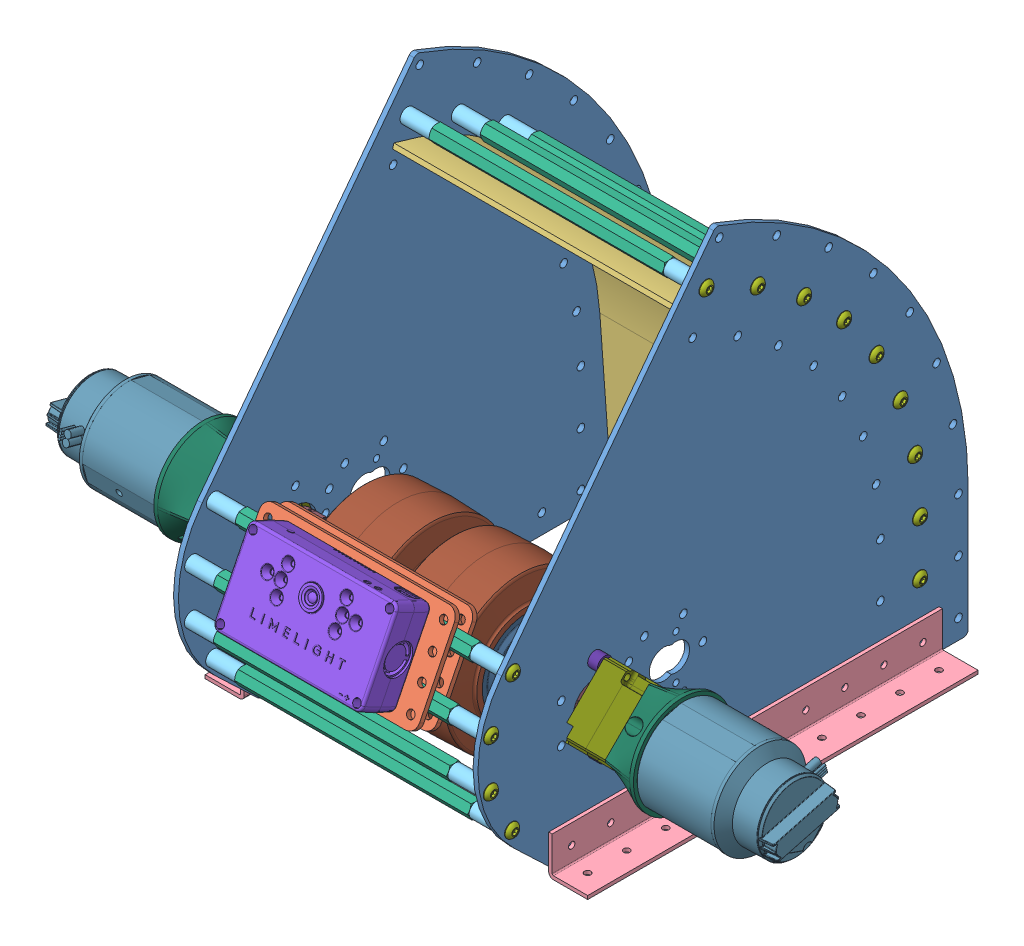
SolidWorks assembly Shooter, configuration Default. Lengths in mm.
Overall size (762 1050.2 1114.79).
114 component instances, 18 part files, 6 mates.
Components (placement in the parent):
- Skeleton-1: Skeleton [Default] at origin
- WCP-0281 Rev1 - GreyT Shooter (Falcon VP Direct)-1: WCP-0281 Rev1 - GreyT Shooter (Falcon VP Direct) [Default] at (-0.625 553.3138 -30.7114) size (474.18 324.22 346.91)
  - frame-GreyT Shooter (Falcon VP Direct)-1: frame-GreyT Shooter (Falcon VP Direct) [Default] at (99.05 0 0) size (248.9 311.77 324.97)
    - WCP-0281-001 Rev1-1: WCP-0281-001 Rev1 [Default] at (-1.5875 82.55 -30.1625) size (3.17 311.77 319.09)
    - WCP-0281-001 Rev1-2: WCP-0281-001 Rev1 [Default] at (-196.5125 82.55 -30.1625) size (3.17 311.77 319.09)
    - WCP-0281-005 Rev1-1: WCP-0281-005 Rev1 [Default] at (-98.4446 110.2154 24.9678) x (1 0 0) z (0 0.446198 0.894934) size (127 63.5 3.17)
    - WCP-0281-005 Rev1-2: WCP-0281-005 Rev1 [Default] at (-98.4446 115.8821 36.3334) x (1 0 0) z (0 0.446198 0.894934) size (127 63.5 3.17)
    - polycarb_flex_panel (WCP-0281-006) Rev1-1: polycarb_flex_panel (WCP-0281-006) Rev1 [Default] at (-97.1926 99.11 -45.232) x (1 0 0) z (0 -0.072501 0.997368) size (184.15 254.67 126.03)
    - WCP-0281-004 Rev1-1: WCP-0281-004 Rev1 [Default] at (0 0 -114.3) size (25.4 25.4 254)
    - WCP-0281-004 Rev1-2: WCP-0281-004 Rev1 [Default] at (-198.1 0 -139.7) x (-1 0 0) z (0 0 -1) size (25.4 25.4 254)
    - spacer_assembly^frame-GreyT Shooter (Falcon VP Direct)-1: spacer_assembly^frame-GreyT Shooter (Falcon VP Direct) [Default] at (-3.8 277.1819 -108.5961) x (1 0 0) z (0 0.167761 -0.985828) size (204.43 13.43 13.43)
      - WCP-0217 Rev1-1: WCP-0217 Rev1 [Default] at (-180.975 -4.7625 -5.4993) x (1 0 0) z (0 -0.707903 0.70631) size (19.05 9.5 9.5)
      - 91780A094_ALUM FEM THRDED HEX STANDOFF (1)_91780A094-1: 91780A094_ALUM FEM THRDED HEX STANDOFF (1)_91780A094 [Default] at (-95.25 -4.7625 -5.4993) x (0 -1 0) z (-1 0 0) size (9.53 11 152.4)
      - WCP-0217 Rev1-2: WCP-0217 Rev1 [Default] at (-9.525 -4.7625 -5.4993) x (1 0 0) z (0 -0.707903 0.70631) size (19.05 9.5 9.5)
      - WCP-0256 Rev1-1: WCP-0256 Rev1 [Default] at (-196.8654 -4.7625 -5.4993) x (0 -0.959732 -0.280918) z (-1 0 0) size (9.24 9.28 34.97)
      - WCP-0256 Rev1-2: WCP-0256 Rev1 [Default] at (6.3654 -4.7625 -5.4993) x (0 0.566489 -0.82407) z (1 0 0) size (9.24 9.28 34.97)
    - spacer_assembly^frame-GreyT Shooter (Falcon VP Direct)-2: spacer_assembly^frame-GreyT Shooter (Falcon VP Direct) [Default] at (-3.8 258.4844 -133.4749) x (1 0 0) z (0 -0.921698 -0.387907) size (204.43 13.43 13.43)
      - WCP-0217 Rev1-1: WCP-0217 Rev1 [Default] at (-180.975 -4.7625 -5.4993) x (1 0 0) z (0 -0.707903 0.70631) size (19.05 9.5 9.5)
      - 91780A094_ALUM FEM THRDED HEX STANDOFF (1)_91780A094-1: 91780A094_ALUM FEM THRDED HEX STANDOFF (1)_91780A094 [Default] at (-95.25 -4.7625 -5.4993) x (0 -1 0) z (-1 0 0) size (9.53 11 152.4)
      - WCP-0217 Rev1-2: WCP-0217 Rev1 [Default] at (-9.525 -4.7625 -5.4993) x (1 0 0) z (0 -0.707903 0.70631) size (19.05 9.5 9.5)
      - WCP-0256 Rev1-1: WCP-0256 Rev1 [Default] at (-196.8654 -4.7625 -5.4993) x (0 -0.959732 -0.280918) z (-1 0 0) size (9.24 9.28 34.97)
      - WCP-0256 Rev1-2: WCP-0256 Rev1 [Default] at (6.3654 -4.7625 -5.4993) x (0 0.566489 -0.82407) z (1 0 0) size (9.24 9.28 34.97)
    - spacer_assembly^frame-GreyT Shooter (Falcon VP Direct)-3: spacer_assembly^frame-GreyT Shooter (Falcon VP Direct) [Default] at (-3.8 237.3746 -163.6227) x (1 0 0) z (0 -0.921698 -0.387907) size (204.43 13.43 13.43)
      - WCP-0217 Rev1-1: WCP-0217 Rev1 [Default] at (-180.975 -4.7625 -5.4993) x (1 0 0) z (0 -0.707903 0.70631) size (19.05 9.5 9.5)
      - 91780A094_ALUM FEM THRDED HEX STANDOFF (1)_91780A094-1: 91780A094_ALUM FEM THRDED HEX STANDOFF (1)_91780A094 [Default] at (-95.25 -4.7625 -5.4993) x (0 -1 0) z (-1 0 0) size (9.53 11 152.4)
      - WCP-0217 Rev1-2: WCP-0217 Rev1 [Default] at (-9.525 -4.7625 -5.4993) x (1 0 0) z (0 -0.707903 0.70631) size (19.05 9.5 9.5)
      - WCP-0256 Rev1-1: WCP-0256 Rev1 [Default] at (-196.8654 -4.7625 -5.4993) x (0 -0.959732 -0.280918) z (-1 0 0) size (9.24 9.28 34.97)
      - WCP-0256 Rev1-2: WCP-0256 Rev1 [Default] at (6.3654 -4.7625 -5.4993) x (0 0.566489 -0.82407) z (1 0 0) size (9.24 9.28 34.97)
    - spacer_assembly^frame-GreyT Shooter (Falcon VP Direct)-4: spacer_assembly^frame-GreyT Shooter (Falcon VP Direct) [Default] at (-3.8 211.3505 -189.6468) x (1 0 0) z (0 -0.921698 -0.387907) size (204.43 13.43 13.43)
      - WCP-0217 Rev1-1: WCP-0217 Rev1 [Default] at (-180.975 -4.7625 -5.4993) x (1 0 0) z (0 -0.707903 0.70631) size (19.05 9.5 9.5)
      - 91780A094_ALUM FEM THRDED HEX STANDOFF (1)_91780A094-1: 91780A094_ALUM FEM THRDED HEX STANDOFF (1)_91780A094 [Default] at (-95.25 -4.7625 -5.4993) x (0 -1 0) z (-1 0 0) size (9.53 11 152.4)
      - WCP-0217 Rev1-2: WCP-0217 Rev1 [Default] at (-9.525 -4.7625 -5.4993) x (1 0 0) z (0 -0.707903 0.70631) size (19.05 9.5 9.5)
      - WCP-0256 Rev1-1: WCP-0256 Rev1 [Default] at (-196.8654 -4.7625 -5.4993) x (0 -0.959732 -0.280918) z (-1 0 0) size (9.24 9.28 34.97)
      - WCP-0256 Rev1-2: WCP-0256 Rev1 [Default] at (6.3654 -4.7625 -5.4993) x (0 0.566489 -0.82407) z (1 0 0) size (9.24 9.28 34.97)
    - spacer_assembly^frame-GreyT Shooter (Falcon VP Direct)-5: spacer_assembly^frame-GreyT Shooter (Falcon VP Direct) [Default] at (-3.8 181.2027 -210.7566) x (1 0 0) z (0 -0.921698 -0.387907) size (204.43 13.43 13.43)
      - WCP-0217 Rev1-1: WCP-0217 Rev1 [Default] at (-180.975 -4.7625 -5.4993) x (1 0 0) z (0 -0.707903 0.70631) size (19.05 9.5 9.5)
      - 91780A094_ALUM FEM THRDED HEX STANDOFF (1)_91780A094-1: 91780A094_ALUM FEM THRDED HEX STANDOFF (1)_91780A094 [Default] at (-95.25 -4.7625 -5.4993) x (0 -1 0) z (-1 0 0) size (9.53 11 152.4)
      - WCP-0217 Rev1-2: WCP-0217 Rev1 [Default] at (-9.525 -4.7625 -5.4993) x (1 0 0) z (0 -0.707903 0.70631) size (19.05 9.5 9.5)
      - WCP-0256 Rev1-1: WCP-0256 Rev1 [Default] at (-196.8654 -4.7625 -5.4993) x (0 -0.959732 -0.280918) z (-1 0 0) size (9.24 9.28 34.97)
      - WCP-0256 Rev1-2: WCP-0256 Rev1 [Default] at (6.3654 -4.7625 -5.4993) x (0 0.566489 -0.82407) z (1 0 0) size (9.24 9.28 34.97)
    - spacer_assembly^frame-GreyT Shooter (Falcon VP Direct)-6: spacer_assembly^frame-GreyT Shooter (Falcon VP Direct) [Default] at (-3.8 147.8472 -226.3105) x (1 0 0) z (0 -0.921698 -0.387907) size (204.43 13.43 13.43)
      - WCP-0217 Rev1-1: WCP-0217 Rev1 [Default] at (-180.975 -4.7625 -5.4993) x (1 0 0) z (0 -0.707903 0.70631) size (19.05 9.5 9.5)
      - 91780A094_ALUM FEM THRDED HEX STANDOFF (1)_91780A094-1: 91780A094_ALUM FEM THRDED HEX STANDOFF (1)_91780A094 [Default] at (-95.25 -4.7625 -5.4993) x (0 -1 0) z (-1 0 0) size (9.53 11 152.4)
      - WCP-0217 Rev1-2: WCP-0217 Rev1 [Default] at (-9.525 -4.7625 -5.4993) x (1 0 0) z (0 -0.707903 0.70631) size (19.05 9.5 9.5)
      - WCP-0256 Rev1-1: WCP-0256 Rev1 [Default] at (-196.8654 -4.7625 -5.4993) x (0 -0.959732 -0.280918) z (-1 0 0) size (9.24 9.28 34.97)
      - WCP-0256 Rev1-2: WCP-0256 Rev1 [Default] at (6.3654 -4.7625 -5.4993) x (0 0.566489 -0.82407) z (1 0 0) size (9.24 9.28 34.97)
    - spacer_assembly^frame-GreyT Shooter (Falcon VP Direct)-7: spacer_assembly^frame-GreyT Shooter (Falcon VP Direct) [Default] at (-3.8 112.2976 -235.836) x (1 0 0) z (0 -0.921698 -0.387907) size (204.43 13.43 13.43)
      - WCP-0217 Rev1-1: WCP-0217 Rev1 [Default] at (-180.975 -4.7625 -5.4993) x (1 0 0) z (0 -0.707903 0.70631) size (19.05 9.5 9.5)
      - 91780A094_ALUM FEM THRDED HEX STANDOFF (1)_91780A094-1: 91780A094_ALUM FEM THRDED HEX STANDOFF (1)_91780A094 [Default] at (-95.25 -4.7625 -5.4993) x (0 -1 0) z (-1 0 0) size (9.53 11 152.4)
      - WCP-0217 Rev1-2: WCP-0217 Rev1 [Default] at (-9.525 -4.7625 -5.4993) x (1 0 0) z (0 -0.707903 0.70631) size (19.05 9.5 9.5)
      - WCP-0256 Rev1-1: WCP-0256 Rev1 [Default] at (-196.8654 -4.7625 -5.4993) x (0 -0.959732 -0.280918) z (-1 0 0) size (9.24 9.28 34.97)
      - WCP-0256 Rev1-2: WCP-0256 Rev1 [Default] at (6.3654 -4.7625 -5.4993) x (0 0.566489 -0.82407) z (1 0 0) size (9.24 9.28 34.97)
    - spacer_assembly^frame-GreyT Shooter (Falcon VP Direct)-8: spacer_assembly^frame-GreyT Shooter (Falcon VP Direct) [Default] at (-3.8 75.6339 -239.0436) x (1 0 0) z (0 -0.921698 -0.387907) size (204.43 13.43 13.43)
      - WCP-0217 Rev1-1: WCP-0217 Rev1 [Default] at (-180.975 -4.7625 -5.4993) x (1 0 0) z (0 -0.707903 0.70631) size (19.05 9.5 9.5)
      - 91780A094_ALUM FEM THRDED HEX STANDOFF (1)_91780A094-1: 91780A094_ALUM FEM THRDED HEX STANDOFF (1)_91780A094 [Default] at (-95.25 -4.7625 -5.4993) x (0 -1 0) z (-1 0 0) size (9.53 11 152.4)
      - WCP-0217 Rev1-2: WCP-0217 Rev1 [Default] at (-9.525 -4.7625 -5.4993) x (1 0 0) z (0 -0.707903 0.70631) size (19.05 9.5 9.5)
      - WCP-0256 Rev1-1: WCP-0256 Rev1 [Default] at (-196.8654 -4.7625 -5.4993) x (0 -0.959732 -0.280918) z (-1 0 0) size (9.24 9.28 34.97)
      - WCP-0256 Rev1-2: WCP-0256 Rev1 [Default] at (6.3654 -4.7625 -5.4993) x (0 0.566489 -0.82407) z (1 0 0) size (9.24 9.28 34.97)
    - spacer_assembly^frame-GreyT Shooter (Falcon VP Direct)-9: spacer_assembly^frame-GreyT Shooter (Falcon VP Direct) [Default] at (-3.8 40.6593 -243.3983) x (1 0 0) z (0 -0.534977 -0.844867) size (204.43 13.43 13.43)
      - WCP-0217 Rev1-1: WCP-0217 Rev1 [Default] at (-180.975 -4.7625 -5.4993) x (1 0 0) z (0 -0.707903 0.70631) size (19.05 9.5 9.5)
      - 91780A094_ALUM FEM THRDED HEX STANDOFF (1)_91780A094-1: 91780A094_ALUM FEM THRDED HEX STANDOFF (1)_91780A094 [Default] at (-95.25 -4.7625 -5.4993) x (0 -1 0) z (-1 0 0) size (9.53 11 152.4)
      - WCP-0217 Rev1-2: WCP-0217 Rev1 [Default] at (-9.525 -4.7625 -5.4993) x (1 0 0) z (0 -0.707903 0.70631) size (19.05 9.5 9.5)
      - WCP-0256 Rev1-1: WCP-0256 Rev1 [Default] at (-196.8654 -4.7625 -5.4993) x (0 -0.959732 -0.280918) z (-1 0 0) size (9.24 9.28 34.97)
      - WCP-0256 Rev1-2: WCP-0256 Rev1 [Default] at (6.3654 -4.7625 -5.4993) x (0 0.566489 -0.82407) z (1 0 0) size (9.24 9.28 34.97)
    - spacer_assembly^frame-GreyT Shooter (Falcon VP Direct)-13: spacer_assembly^frame-GreyT Shooter (Falcon VP Direct) [Default] at (-3.8 119.8597 24.594) x (1 0 0) z (0 -0.833886 -0.551937) size (204.43 13.43 13.43)
      - WCP-0217 Rev1-1: WCP-0217 Rev1 [Default] at (-180.975 -4.7625 -5.4993) x (1 0 0) z (0 -0.707903 0.70631) size (19.05 9.5 9.5)
      - 91780A094_ALUM FEM THRDED HEX STANDOFF (1)_91780A094-1: 91780A094_ALUM FEM THRDED HEX STANDOFF (1)_91780A094 [Default] at (-95.25 -4.7625 -5.4993) x (0 -1 0) z (-1 0 0) size (9.53 11 152.4)
      - WCP-0217 Rev1-2: WCP-0217 Rev1 [Default] at (-9.525 -4.7625 -5.4993) x (1 0 0) z (0 -0.707903 0.70631) size (19.05 9.5 9.5)
      - WCP-0256 Rev1-1: WCP-0256 Rev1 [Default] at (-196.8654 -4.7625 -5.4993) x (0 -0.959732 -0.280918) z (-1 0 0) size (9.24 9.28 34.97)
      - WCP-0256 Rev1-2: WCP-0256 Rev1 [Default] at (6.3654 -4.7625 -5.4993) x (0 0.566489 -0.82407) z (1 0 0) size (9.24 9.28 34.97)
    - spacer_assembly^frame-GreyT Shooter (Falcon VP Direct)-14: spacer_assembly^frame-GreyT Shooter (Falcon VP Direct) [Default] at (-3.8 91.5232 38.722) x (1 0 0) z (0 -0.833886 -0.551937) size (204.43 13.43 13.43)
      - WCP-0217 Rev1-1: WCP-0217 Rev1 [Default] at (-180.975 -4.7625 -5.4993) x (1 0 0) z (0 -0.707903 0.70631) size (19.05 9.5 9.5)
      - 91780A094_ALUM FEM THRDED HEX STANDOFF (1)_91780A094-1: 91780A094_ALUM FEM THRDED HEX STANDOFF (1)_91780A094 [Default] at (-95.25 -4.7625 -5.4993) x (0 -1 0) z (-1 0 0) size (9.53 11 152.4)
      - WCP-0217 Rev1-2: WCP-0217 Rev1 [Default] at (-9.525 -4.7625 -5.4993) x (1 0 0) z (0 -0.707903 0.70631) size (19.05 9.5 9.5)
      - WCP-0256 Rev1-1: WCP-0256 Rev1 [Default] at (-196.8654 -4.7625 -5.4993) x (0 -0.959732 -0.280918) z (-1 0 0) size (9.24 9.28 34.97)
      - WCP-0256 Rev1-2: WCP-0256 Rev1 [Default] at (6.3654 -4.7625 -5.4993) x (0 0.566489 -0.82407) z (1 0 0) size (9.24 9.28 34.97)
    - spacer_assembly^frame-GreyT Shooter (Falcon VP Direct)-15: spacer_assembly^frame-GreyT Shooter (Falcon VP Direct) [Default] at (-3.8 59.8605 38.8878) x (1 0 0) z (0 -0.833886 -0.551937) size (204.43 13.43 13.43)
      - WCP-0217 Rev1-1: WCP-0217 Rev1 [Default] at (-180.975 -4.7625 -5.4993) x (1 0 0) z (0 -0.707903 0.70631) size (19.05 9.5 9.5)
      - 91780A094_ALUM FEM THRDED HEX STANDOFF (1)_91780A094-1: 91780A094_ALUM FEM THRDED HEX STANDOFF (1)_91780A094 [Default] at (-95.25 -4.7625 -5.4993) x (0 -1 0) z (-1 0 0) size (9.53 11 152.4)
      - WCP-0217 Rev1-2: WCP-0217 Rev1 [Default] at (-9.525 -4.7625 -5.4993) x (1 0 0) z (0 -0.707903 0.70631) size (19.05 9.5 9.5)
      - WCP-0256 Rev1-1: WCP-0256 Rev1 [Default] at (-196.8654 -4.7625 -5.4993) x (0 -0.959732 -0.280918) z (-1 0 0) size (9.24 9.28 34.97)
      - WCP-0256 Rev1-2: WCP-0256 Rev1 [Default] at (6.3654 -4.7625 -5.4993) x (0 0.566489 -0.82407) z (1 0 0) size (9.24 9.28 34.97)
    - spacer_assembly^frame-GreyT Shooter (Falcon VP Direct)-16: spacer_assembly^frame-GreyT Shooter (Falcon VP Direct) [Default] at (-3.8 31.3776 25.0573) x (1 0 0) z (0 -0.833886 -0.551937) size (204.43 13.43 13.43)
      - WCP-0217 Rev1-1: WCP-0217 Rev1 [Default] at (-180.975 -4.7625 -5.4993) x (1 0 0) z (0 -0.707903 0.70631) size (19.05 9.5 9.5)
      - 91780A094_ALUM FEM THRDED HEX STANDOFF (1)_91780A094-1: 91780A094_ALUM FEM THRDED HEX STANDOFF (1)_91780A094 [Default] at (-95.25 -4.7625 -5.4993) x (0 -1 0) z (-1 0 0) size (9.53 11 152.4)
      - WCP-0217 Rev1-2: WCP-0217 Rev1 [Default] at (-9.525 -4.7625 -5.4993) x (1 0 0) z (0 -0.707903 0.70631) size (19.05 9.5 9.5)
      - WCP-0256 Rev1-1: WCP-0256 Rev1 [Default] at (-196.8654 -4.7625 -5.4993) x (0 -0.959732 -0.280918) z (-1 0 0) size (9.24 9.28 34.97)
      - WCP-0256 Rev1-2: WCP-0256 Rev1 [Default] at (6.3654 -4.7625 -5.4993) x (0 0.566489 -0.82407) z (1 0 0) size (9.24 9.28 34.97)
  - LimelightCAD2STEPSimp-1: LimelightCAD2STEPSimp [Default] at (9.23 125.4056 67.1857) x (1 0 0) z (0 -0.894934 0.446198) size (97.88 26.09 57.01)
  - flywheel_assembly - GreyT Shooter (Falcon VP Direct)-2: flywheel_assembly - GreyT Shooter (Falcon VP Direct) [Default] at (0 84.6779 -8.3849) x (1 0 0) z (0 0.587407 -0.809292) size (127 136.01 136.01)
    - flywheel_bar - GreyT Shooter (Falcon VP Direct)-1: flywheel_bar - GreyT Shooter (Falcon VP Direct) [Default] at (0 14.5144 16.3745) size (127 12.7 13.75)
      - WCP-0281-007 Rev1-1: WCP-0281-007 Rev1 [Default] at origin size (127 12.7 13.75)
    - 2in_flywheel_w_hex (217-4054)-1: 2in_flywheel_w_hex (217-4054) [Default] at (-28.9766 14.5144 16.3598) x (1 0 0) z (0 0.866025 0.5) size (57.95 99.57 99.57)
      - 217-4054-003 Rev1-1: 217-4054-003 Rev1 [Default] at origin size (55.55 82.55 82.55)
      - 217-4054-004 Rev1-1: 217-4054-004 Rev1 [Default] at origin size (50.8 99.57 99.57)
      - 217-4054-002 Rev15-1: 217-4054-002 Rev15 [Default] x (0 0 1) z (-1 0 0) size (50.79 50.79 57.95)
    - 2in_flywheel_w_hex (217-4054)-2: 2in_flywheel_w_hex (217-4054) [Default] at (28.9766 14.5398 16.3745) size (57.95 99.57 99.57)
      - 217-4054-003 Rev1-1: 217-4054-003 Rev1 [Default] at origin size (55.55 82.55 82.55)
      - 217-4054-004 Rev1-1: 217-4054-004 Rev1 [Default] at origin size (50.8 99.57 99.57)
      - 217-4054-002 Rev15-1: 217-4054-002 Rev15 [Default] x (0 0 1) z (-1 0 0) size (50.79 50.79 57.95)
  - turret_motor_assembly (Falcon VP Direct)-3: turret_motor_assembly (Falcon VP Direct) [Default] at (-6.975 82.55 -30.1625) x (-1 0 0) z (0 0 -1) size (180.04 90.51 90.51)
    - 217-4008_500_Hex_Coupler-1: 217-4008_500_Hex_Coupler [Default] at (69.85 0 0) x (0 -0.407164 -0.913355) z (1 0 0) size (25.38 22.32 39.56)
    - 217-6515_Falcon_500_Default_As Machined_-1: 217-6515_Falcon_500_Default_As Machined_ [Default] at (175.3 0 0) x (0 0.965926 -0.258819) z (-1 0 0) size (63.31 63.31 115.82)
    - 217-4018_VersaPlanetary_CIM_Adapter-1: 217-4018_VersaPlanetary_CIM_Adapter [Default] at (137.575 0 0) x (0 -0.707107 -0.707107) z (0 0.707107 -0.707107) size (64 21.67 64)
    - v2_versa_planetary_1_stage_no_motor-1: v2_versa_planetary_1_stage_no_motor [Default] at (115.05 -15.7154 15.7154) x (-1 0 0) z (0 -0.707107 -0.707107) size (91.96 44.45 42)
    - WCP-0308-1: WCP-0308 [Default] at (95.25 25.4 0) size (6.35 9.5 9.5)
    - WCP-0308-2: WCP-0308 [Default] at (95.25 -25.4 0) size (6.35 9.5 9.5)
  - turret_motor_assembly (Falcon VP Direct)-4: turret_motor_assembly (Falcon VP Direct) [Default] at (6.975 82.55 -30.1625) size (180.04 90.51 90.51)
    - 217-4008_500_Hex_Coupler-1: 217-4008_500_Hex_Coupler [Default] at (69.85 0 0) x (0 -0.407164 -0.913355) z (1 0 0) size (25.38 22.32 39.56)
    - 217-6515_Falcon_500_Default_As Machined_-1: 217-6515_Falcon_500_Default_As Machined_ [Default] at (175.3 0 0) x (0 0.965926 -0.258819) z (-1 0 0) size (63.31 63.31 115.82)
    - 217-4018_VersaPlanetary_CIM_Adapter-1: 217-4018_VersaPlanetary_CIM_Adapter [Default] at (137.575 0 0) x (0 -0.707107 -0.707107) z (0 0.707107 -0.707107) size (64 21.67 64)
    - v2_versa_planetary_1_stage_no_motor-1: v2_versa_planetary_1_stage_no_motor [Default] at (115.05 -15.7154 15.7154) x (-1 0 0) z (0 -0.707107 -0.707107) size (91.96 44.45 42)
    - WCP-0308-1: WCP-0308 [Default] at (95.25 25.4 0) size (6.35 9.5 9.5)
    - WCP-0308-2: WCP-0308 [Default] at (95.25 -25.4 0) size (6.35 9.5 9.5)
Mates (geometry in assembly coordinates):
- Coincident2: coincident aligned: plane of Skeleton-1 through (0 0 0) normal (0 0 1)
- Coincident3: coincident aligned: plane of Skeleton-1 through (0 0 0) normal (0 1 0)
- Coincident4: coincident aligned: plane of Skeleton-1 through (0 0 0) normal (1 0 0)
- Coincident5: coincident anti-aligned: plane of Skeleton-1 through (0 553.3138 0) normal (0 1 0); plane of WCP-0281 Rev1 - GreyT Shooter (Falcon VP Direct)-1/frame-GreyT Shooter (Falcon VP Direct)-1/WCP-0281-004 Rev1-1 through (98.425 553.3138 -894.3114) normal (0 -1 0)
- Coincident6: coincident: line of Skeleton-1 through (123.825 553.3138 -30.7114) axis (0 0 -1); plane of WCP-0281 Rev1 - GreyT Shooter (Falcon VP Direct)-1/frame-GreyT Shooter (Falcon VP Direct)-1/WCP-0281-004 Rev1-1 through (123.825 555.5998 -894.3114) normal (1 0 0)
- Coincident7: coincident: line of Skeleton-1 through (-123.825 553.3138 -30.7114) axis (1 0 0); plane of WCP-0281 Rev1 - GreyT Shooter (Falcon VP Direct)-1/frame-GreyT Shooter (Falcon VP Direct)-1/WCP-0281-004 Rev1-1 through (96.9391 553.3138 -30.7114) normal (0 0 1)
